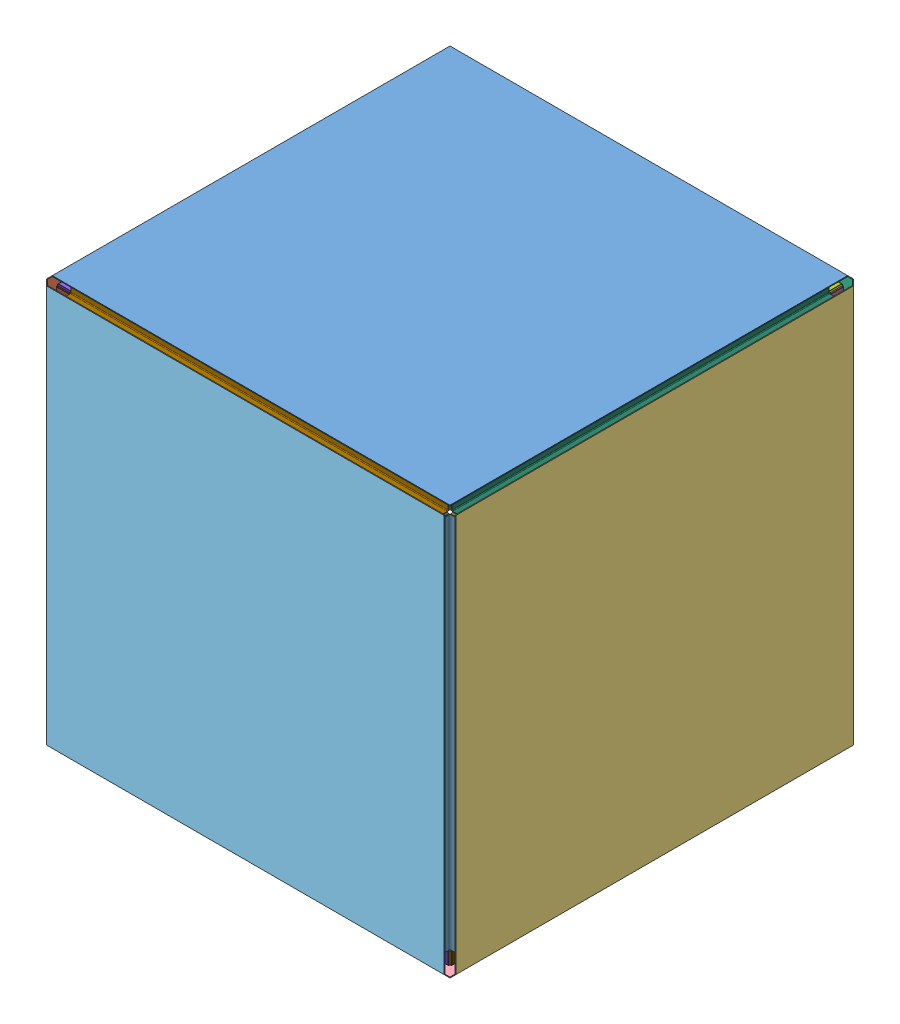
SolidWorks assembly cube_31, configuration cube31. Lengths in mm.
Overall size (770.25 770.25 770.25).
30 component instances, 30 part files, 93 mates.
Components (placement in the parent):
- pr^cube_31-28: pr^cube_31 [cube01] x (-1 0 0) z (0 0 1) size (748.03 1.59 748.03) (virtual)
- pg^cube_31-20: pg^cube_31 [cube01] x (0 -1 0) z (0 0 1) size (748.03 1.59 748.03) (virtual)
- po^cube_31-22: po^cube_31 [cube01] x (0 1 0) z (0 0 1) size (748.03 1.59 748.03) (virtual)
- py^cube_31-21: py^cube_31 [cube01] at origin size (748.03 1.59 748.03) (virtual)
- pc^cube_31-18: pc^cube_31 [cube01] x (-1 0 0) z (0 -1 0) size (748.03 1.59 748.03) (virtual)
- pb^cube_31-21: pb^cube_31 [cube01] x (-1 0 0) z (0 1 0) size (748.03 1.59 748.03) (virtual)
- br1^cube_31-49: br1^cube_31 [Default] at (0 358.14 -358.14) x (0 0 1) z (-1 0 0) size (50.8 50.8 709.17) (virtual)
- br2^cube_31-61: br2^cube_31 [Default] at (-358.14 358.14 0) size (50.8 50.8 709.17) (virtual)
- br3^cube_31-46: br3^cube_31 [Default] at (0 358.14 358.14) x (0 0 -1) z (1 0 0) size (50.8 50.8 709.17) (virtual)
- bg1^cube_31-47: bg1^cube_31 [Default] at (-358.14 -358.14 0) x (0 1 0) z (0 0 1) size (50.8 50.8 709.17) (virtual)
- bg2^cube_31-44: bg2^cube_31 [Default] at (-358.14 0 358.14) x (0 0 -1) z (0 1 0) size (50.8 50.8 709.17) (virtual)
- bg3^cube_31-40: bg3^cube_31 [Default] at (-358.14 0 -358.14) x (0 0 1) z (0 -1 0) size (50.8 50.8 709.17) (virtual)
- bo1^cube_31-42: bo1^cube_31 [Default] at (358.14 0 -358.14) x (0 0 1) z (0 1 0) size (50.8 50.8 709.17) (virtual)
- bo2^cube_31-46: bo2^cube_31 [Default] at (358.14 0 358.14) x (0 0 -1) z (0 -1 0) size (50.8 50.8 709.17) (virtual)
- bo3^cube_31-62: bo3^cube_31 [Default] at (358.14 358.14 0) x (0 -1 0) z (0 0 1) size (50.8 50.8 709.17) (virtual)
- by1^cube_31-41: by1^cube_31 [Default] at (0 -358.14 -358.14) x (0 0 1) z (1 0 0) size (50.8 50.8 709.17) (virtual)
- by2^cube_31-45: by2^cube_31 [Default] at (0 -358.14 358.14) x (0 0 -1) z (-1 0 0) size (50.8 50.8 709.17) (virtual)
- by3^cube_31-48: by3^cube_31 [Default] at (358.14 -358.14 0) x (-1 0 0) z (0 0 1) size (50.8 50.8 709.17) (virtual)
- dr1^cube_31-55: dr1^cube_31 [cube01] at (-382.9346 383.54 0) x (0 -1 0) z (0 0 1) size (26.01 26.01 767.09) (hidden, virtual)
- dr2^cube_31-37: dr2^cube_31 [cube01] at (0 383.54 382.9346) x (0 -1 0) z (1 0 0) size (26.01 26.01 767.09) (hidden, virtual)
- dr3^cube_31-33: dr3^cube_31 [cube01] at (0 383.54 -382.9346) x (0 -1 0) z (-1 0 0) size (26.01 26.01 767.09) (hidden, virtual)
- dg1^cube_31-38: dg1^cube_31 [cube01] at (-383.54 0 382.9346) x (1 0 0) z (0 1 0) size (26.01 26.01 767.09) (hidden, virtual)
- dg2^cube_31-41: dg2^cube_31 [cube01] at (-383.54 -382.9346 0) size (26.01 26.01 767.09) (hidden, virtual)
- dg3^cube_31-34: dg3^cube_31 [cube01] at (-383.54 0 -382.9346) x (1 0 0) z (0 -1 0) size (26.01 26.01 767.09) (hidden, virtual)
- do3^cube_31-47: do3^cube_31 [cube01] at (383.54 382.9346 0) x (-1 0 0) z (0 0 1) size (26.01 26.01 767.09) (hidden, virtual)
- do1^cube_31-36: do1^cube_31 [cube01] at (383.54 0 -382.9346) x (-1 0 0) z (0 1 0) size (26.01 26.01 767.09) (hidden, virtual)
- do2^cube_31-40: do2^cube_31 [cube01] at (383.54 0 382.9346) x (-1 0 0) z (0 -1 0) size (26.01 26.01 767.09) (hidden, virtual)
- dy1^cube_31-35: dy1^cube_31 [cube01] at (0 -383.54 -382.9346) x (0 1 0) z (1 0 0) size (26.01 26.01 767.09) (hidden, virtual)
- dy2^cube_31-39: dy2^cube_31 [cube01] at (0 -383.54 382.9346) x (0 1 0) z (-1 0 0) size (26.01 26.01 767.09) (hidden, virtual)
- dy3^cube_31-42: dy3^cube_31 [cube01] at (382.9346 -383.54 0) x (0 1 0) z (0 0 1) size (26.01 26.01 767.09) (hidden, virtual)
Mates (geometry in assembly coordinates):
- Coincident1: coincident anti-aligned: plane of pr^cube_31-28 through (374.015 383.54 -374.015) normal (0 -1 0); plane of br1^cube_31-49 through (-354.584 383.54 -358.14) normal (0 1 0)
- Coincident2: coincident anti-aligned: plane of pr^cube_31-28 through (374.015 383.54 -374.015) normal (0 -1 0); plane of br2^cube_31-61 through (-358.14 383.54 354.584) normal (0 1 0)
- Coincident3: coincident anti-aligned: plane of pr^cube_31-28 through (374.015 383.54 -374.015) normal (0 -1 0); plane of br3^cube_31-46 through (354.584 383.54 358.14) normal (0 1 0)
- Coincident4: coincident anti-aligned: plane of pr^cube_31-28 through (374.015 383.54 -374.015) normal (0 -1 0); plane of bo3^cube_31-62 through (358.14 383.54 354.584) normal (0 1 0)
- Coincident5: coincident anti-aligned: plane of pr^cube_31-28 through (374.015 383.54 -374.015) normal (0 -1 0); plane of dr3^cube_31-33 through (0 383.54 -766.4746) normal (0 1 0)
- Coincident6: coincident anti-aligned: plane of pr^cube_31-28 through (374.015 383.54 -374.015) normal (0 -1 0); plane of dr1^cube_31-55 through (-766.4746 383.54 0) normal (0 1 0)
- Coincident7: coincident anti-aligned: plane of pr^cube_31-28 through (374.015 383.54 -374.015) normal (0 -1 0); plane of do3^cube_31-47 through (-0.6054 383.54 0) normal (0 1 0)
- Coincident8: coincident anti-aligned: plane of pr^cube_31-28 through (374.015 383.54 -374.015) normal (0 -1 0); plane of dr2^cube_31-37 through (0 383.54 766.4746) normal (0 1 0)
- Coincident34: coincident anti-aligned: plane of pb^cube_31-21 through (374.015 -374.015 -383.54) normal (0 0 1); plane of by1^cube_31-41 through (354.584 -358.14 -383.54) normal (0 0 -1)
- Coincident35: coincident anti-aligned: plane of pb^cube_31-21 through (374.015 -374.015 -383.54) normal (0 0 1); plane of bo1^cube_31-42 through (358.14 354.584 -383.54) normal (0 0 -1)
- Coincident36: coincident anti-aligned: plane of pb^cube_31-21 through (374.015 -374.015 -383.54) normal (0 0 1); plane of br1^cube_31-49 through (-354.584 358.14 -383.54) normal (0 0 -1)
- Coincident37: coincident anti-aligned: plane of pb^cube_31-21 through (374.015 -374.015 -383.54) normal (0 0 1); plane of bg3^cube_31-40 through (-358.14 -354.584 -383.54) normal (0 0 -1)
- Coincident38: coincident anti-aligned: plane of pb^cube_31-21 through (374.015 -374.015 -383.54) normal (0 0 1); plane of dg3^cube_31-34 through (0.6054 0 -383.54) normal (0 0 -1)
- Coincident39: coincident anti-aligned: plane of pb^cube_31-21 through (374.015 -374.015 -383.54) normal (0 0 1); plane of dr3^cube_31-33 through (0 -0.6054 -383.54) normal (0 0 -1)
- Coincident40: coincident anti-aligned: plane of pb^cube_31-21 through (374.015 -374.015 -383.54) normal (0 0 1); plane of do1^cube_31-36 through (-0.6054 0 -383.54) normal (0 0 -1)
- Coincident41: coincident anti-aligned: plane of pb^cube_31-21 through (374.015 -374.015 -383.54) normal (0 0 1); plane of dy1^cube_31-35 through (0 0.6054 -383.54) normal (0 0 -1)
- Coincident42: coincident anti-aligned: plane of pc^cube_31-18 through (374.015 374.015 383.54) normal (0 0 -1); plane of bo2^cube_31-46 through (358.14 -354.584 383.54) normal (0 0 1)
- Coincident43: coincident anti-aligned: plane of pc^cube_31-18 through (374.015 374.015 383.54) normal (0 0 -1); plane of br3^cube_31-46 through (354.584 358.14 383.54) normal (0 0 1)
- Coincident44: coincident anti-aligned: plane of pc^cube_31-18 through (374.015 374.015 383.54) normal (0 0 -1); plane of bg2^cube_31-44 through (-358.14 354.584 383.54) normal (0 0 1)
- Coincident45: coincident anti-aligned: plane of pc^cube_31-18 through (374.015 374.015 383.54) normal (0 0 -1); plane of by2^cube_31-45 through (-354.584 -358.14 383.54) normal (0 0 1)
- Coincident46: coincident anti-aligned: plane of pc^cube_31-18 through (374.015 374.015 383.54) normal (0 0 -1); plane of do2^cube_31-40 through (-0.6054 0 383.54) normal (0 0 1)
- Coincident47: coincident anti-aligned: plane of pc^cube_31-18 through (374.015 374.015 383.54) normal (0 0 -1); plane of dy2^cube_31-39 through (0 0.6054 383.54) normal (0 0 1)
- Coincident48: coincident anti-aligned: plane of pc^cube_31-18 through (374.015 374.015 383.54) normal (0 0 -1); plane of dg1^cube_31-38 through (0.6054 0 383.54) normal (0 0 1)
- Coincident49: coincident anti-aligned: plane of pc^cube_31-18 through (374.015 374.015 383.54) normal (0 0 -1); plane of dr2^cube_31-37 through (0 -0.6054 383.54) normal (0 0 1)
- Coincident50: coincident anti-aligned: plane of pg^cube_31-20 through (-383.54 374.015 -374.015) normal (1 0 0); plane of bg3^cube_31-40 through (-383.54 -354.584 -358.14) normal (-1 0 0)
- Coincident51: coincident anti-aligned: plane of pg^cube_31-20 through (-383.54 374.015 -374.015) normal (1 0 0); plane of bg1^cube_31-47 through (-383.54 -358.14 354.584) normal (-1 0 0)
- Coincident52: coincident anti-aligned: plane of pg^cube_31-20 through (-383.54 374.015 -374.015) normal (1 0 0); plane of bg2^cube_31-44 through (-383.54 354.584 358.14) normal (-1 0 0)
- Coincident53: coincident anti-aligned: plane of pg^cube_31-20 through (-383.54 374.015 -374.015) normal (1 0 0); plane of dr1^cube_31-55 through (-383.54 -0.6054 0) normal (-1 0 0)
- Coincident54: coincident anti-aligned: plane of pg^cube_31-20 through (-383.54 374.015 -374.015) normal (1 0 0); plane of dg3^cube_31-34 through (-383.54 0 -766.4746) normal (-1 0 0)
- Coincident55: coincident anti-aligned: plane of pg^cube_31-20 through (-383.54 374.015 -374.015) normal (1 0 0); plane of dg2^cube_31-41 through (-383.54 -766.4746 0) normal (-1 0 0)
- Coincident56: coincident anti-aligned: plane of pg^cube_31-20 through (-383.54 374.015 -374.015) normal (1 0 0); plane of dg1^cube_31-38 through (-383.54 0 766.4746) normal (-1 0 0)
- Coincident99: coincident anti-aligned: plane of pg^cube_31-20 through (-383.54 374.015 -374.015) normal (1 0 0); plane of br2^cube_31-61 through (-383.54 358.14 354.584) normal (-1 0 0)
- Coincident57: coincident anti-aligned: plane of py^cube_31-21 through (-374.015 -383.54 -374.015) normal (0 1 0); plane of by3^cube_31-48 through (358.14 -383.54 354.584) normal (0 -1 0)
- Coincident58: coincident anti-aligned: plane of py^cube_31-21 through (-374.015 -383.54 -374.015) normal (0 1 0); plane of by2^cube_31-45 through (-354.584 -383.54 358.14) normal (0 -1 0)
- Coincident59: coincident anti-aligned: plane of py^cube_31-21 through (-374.015 -383.54 -374.015) normal (0 1 0); plane of bg1^cube_31-47 through (-358.14 -383.54 354.584) normal (0 -1 0)
- Coincident60: coincident anti-aligned: plane of py^cube_31-21 through (-374.015 -383.54 -374.015) normal (0 1 0); plane of by1^cube_31-41 through (354.584 -383.54 -358.14) normal (0 -1 0)
- Coincident61: coincident anti-aligned: plane of py^cube_31-21 through (-374.015 -383.54 -374.015) normal (0 1 0); plane of dy3^cube_31-42 through (766.4746 -383.54 0) normal (0 -1 0)
- Coincident62: coincident anti-aligned: plane of py^cube_31-21 through (-374.015 -383.54 -374.015) normal (0 1 0); plane of dy2^cube_31-39 through (0 -383.54 766.4746) normal (0 -1 0)
- Coincident63: coincident anti-aligned: plane of py^cube_31-21 through (-374.015 -383.54 -374.015) normal (0 1 0); plane of dg2^cube_31-41 through (0.6054 -383.54 0) normal (0 -1 0)
- Coincident64: coincident anti-aligned: plane of py^cube_31-21 through (-374.015 -383.54 -374.015) normal (0 1 0); plane of dy1^cube_31-35 through (0 -383.54 -766.4746) normal (0 -1 0)
- Coincident65: coincident anti-aligned: plane of po^cube_31-22 through (383.54 -374.015 -374.015) normal (-1 0 0); plane of bo1^cube_31-42 through (383.54 354.584 -358.14) normal (1 0 0)
- Coincident66: coincident anti-aligned: plane of po^cube_31-22 through (383.54 -374.015 -374.015) normal (-1 0 0); plane of by3^cube_31-48 through (383.54 -358.14 354.584) normal (1 0 0)
- Coincident67: coincident anti-aligned: plane of po^cube_31-22 through (383.54 -374.015 -374.015) normal (-1 0 0); plane of bo2^cube_31-46 through (383.54 -354.584 358.14) normal (1 0 0)
- Coincident68: coincident anti-aligned: plane of po^cube_31-22 through (383.54 -374.015 -374.015) normal (-1 0 0); plane of bo3^cube_31-62 through (383.54 358.14 354.584) normal (1 0 0)
- Coincident69: coincident anti-aligned: plane of po^cube_31-22 through (383.54 -374.015 -374.015) normal (-1 0 0); plane of do2^cube_31-40 through (383.54 0 766.4746) normal (1 0 0)
- Coincident70: coincident anti-aligned: plane of po^cube_31-22 through (383.54 -374.015 -374.015) normal (-1 0 0); plane of do3^cube_31-47 through (383.54 766.4746 0) normal (1 0 0)
- Coincident71: coincident anti-aligned: plane of po^cube_31-22 through (383.54 -374.015 -374.015) normal (-1 0 0); plane of do1^cube_31-36 through (383.54 0 -766.4746) normal (1 0 0)
- Coincident72: coincident anti-aligned: plane of po^cube_31-22 through (383.54 -374.015 -374.015) normal (-1 0 0); plane of dy3^cube_31-42 through (383.54 0.6054 0) normal (1 0 0)
- Coincident73: coincident aligned: plane of assembly through (0 0 0) normal (0 0 1); plane of dy3^cube_31-42 through (382.9346 -383.54 0) normal (0 0 1)
- Coincident74: coincident aligned: plane of assembly through (0 0 0) normal (0 0 1); plane of by3^cube_31-48 through (358.14 -358.14 0) normal (0 0 1)
- Coincident75: coincident aligned: plane of assembly through (0 0 0) normal (0 0 1); plane of bo3^cube_31-62 through (358.14 358.14 0) normal (0 0 1)
- Coincident76: coincident aligned: plane of assembly through (0 0 0) normal (0 0 1); plane of do3^cube_31-47 through (383.54 382.9346 0) normal (0 0 1)
- Coincident77: coincident aligned: plane of assembly through (0 0 0) normal (0 0 1); plane of dg2^cube_31-41 through (-383.54 -382.9346 0) normal (0 0 1)
- Coincident78: coincident aligned: plane of assembly through (0 0 0) normal (0 0 1); plane of bg1^cube_31-47 through (-358.14 -358.14 0) normal (0 0 1)
- Coincident79: coincident aligned: plane of assembly through (0 0 0) normal (0 0 1); plane of dr1^cube_31-55 through (-382.9346 383.54 0) normal (0 0 1)
- Coincident80: coincident aligned: plane of assembly through (0 0 0) normal (0 0 1); plane of br2^cube_31-61 through (-358.14 358.14 0) normal (0 0 1)
- Coincident81: coincident aligned: plane of assembly through (0 0 0) normal (0 1 0); plane of bo1^cube_31-42 through (358.14 0 -358.14) normal (0 1 0)
- Coincident82: coincident aligned: plane of assembly through (0 0 0) normal (0 1 0); plane of py^cube_31-21 through (0 0 0) normal (0 1 0)
- Coincident83: coincident aligned: plane of assembly through (0 0 0) normal (0 1 0); plane of do1^cube_31-36 through (383.54 0 -382.9346) normal (0 1 0)
- Coincident84: coincident anti-aligned: plane of assembly through (0 0 0) normal (0 1 0); plane of bg3^cube_31-40 through (-358.14 0 -358.14) normal (0 -1 0)
- Coincident85: coincident anti-aligned: plane of assembly through (0 0 0) normal (0 1 0); plane of dg3^cube_31-34 through (-383.54 0 -382.9346) normal (0 -1 0)
- Coincident86: coincident aligned: plane of assembly through (0 0 0) normal (0 1 0); plane of dg1^cube_31-38 through (-383.54 0 382.9346) normal (0 1 0)
- Coincident87: coincident aligned: plane of assembly through (0 0 0) normal (0 1 0); plane of bg2^cube_31-44 through (-358.14 0 358.14) normal (0 1 0)
- Coincident88: coincident anti-aligned: plane of assembly through (0 0 0) normal (0 1 0); plane of bo2^cube_31-46 through (358.14 0 358.14) normal (0 -1 0)
- Coincident89: coincident anti-aligned: plane of assembly through (0 0 0) normal (0 1 0); plane of do2^cube_31-40 through (383.54 0 382.9346) normal (0 -1 0)
- Coincident90: coincident anti-aligned: plane of assembly through (0 0 0) normal (1 0 0); plane of by2^cube_31-45 through (0 -358.14 358.14) normal (-1 0 0)
- Coincident91: coincident anti-aligned: plane of assembly through (0 0 0) normal (1 0 0); plane of dy2^cube_31-39 through (0 -383.54 382.9346) normal (-1 0 0)
- Coincident92: coincident aligned: plane of assembly through (0 0 0) normal (1 0 0); plane of pg^cube_31-20
- Coincident93: coincident aligned: plane of assembly through (0 0 0) normal (1 0 0); plane of dr2^cube_31-37 through (0 383.54 382.9346) normal (1 0 0)
- Coincident94: coincident aligned: plane of assembly through (0 0 0) normal (1 0 0); plane of br3^cube_31-46 through (0 358.14 358.14) normal (1 0 0)
- Coincident95: coincident anti-aligned: plane of assembly through (0 0 0) normal (1 0 0); plane of dr3^cube_31-33 through (0 383.54 -382.9346) normal (-1 0 0)
- Coincident96: coincident anti-aligned: plane of assembly through (0 0 0) normal (1 0 0); plane of br1^cube_31-49 through (0 358.14 -358.14) normal (-1 0 0)
- Coincident97: coincident aligned: plane of assembly through (0 0 0) normal (1 0 0); plane of by1^cube_31-41 through (0 -358.14 -358.14) normal (1 0 0)
- Coincident98: coincident aligned: plane of assembly through (0 0 0) normal (1 0 0); plane of dy1^cube_31-35 through (0 -383.54 -382.9346) normal (1 0 0)
- Coincident100: coincident anti-aligned: plane of pr^cube_31-28; plane of assembly through (0 0 0) normal (1 0 0)
- Coincident101: coincident aligned: plane of pr^cube_31-28 through (0 0 0) normal (0 0 1); plane of assembly through (0 0 0) normal (0 0 1)
- Coincident102: coincident anti-aligned: plane of pr^cube_31-28; plane of assembly through (0 0 0) normal (0 1 0)
- Coincident106: coincident anti-aligned: plane of pg^cube_31-20; plane of assembly through (0 0 0) normal (0 1 0)
- Coincident107: coincident aligned: plane of pg^cube_31-20; plane of assembly through (0 0 0) normal (1 0 0)
- Coincident108: coincident aligned: plane of pg^cube_31-20 through (0 0 0) normal (0 0 1); plane of assembly through (0 0 0) normal (0 0 1)
- Coincident109: coincident aligned: plane of py^cube_31-21 through (0 0 0) normal (0 0 1); plane of assembly through (0 0 0) normal (0 0 1)
- Coincident110: coincident aligned: plane of py^cube_31-21 through (0 0 0) normal (0 1 0); plane of assembly through (0 0 0) normal (0 1 0)
- Coincident111: coincident aligned: plane of py^cube_31-21 through (0 0 0) normal (1 0 0); plane of assembly through (0 0 0) normal (1 0 0)
- Coincident112: coincident aligned: plane of po^cube_31-22 through (0 0 0) normal (0 0 1); plane of assembly through (0 0 0) normal (0 0 1)
- Coincident113: coincident anti-aligned: plane of po^cube_31-22; plane of assembly through (0 0 0) normal (1 0 0)
- Coincident114: coincident aligned: plane of po^cube_31-22; plane of assembly through (0 0 0) normal (0 1 0)
- Coincident115: coincident anti-aligned: plane of pc^cube_31-18 through (0 0 0) normal (0 -1 0); plane of assembly through (0 0 0) normal (0 1 0)
- Coincident116: coincident anti-aligned: plane of pc^cube_31-18; plane of assembly through (0 0 0) normal (0 0 1)
- Coincident117: coincident anti-aligned: plane of pc^cube_31-18; plane of assembly through (0 0 0) normal (1 0 0)
- Coincident118: coincident aligned: plane of pb^cube_31-21 through (0 0 0) normal (0 1 0); plane of assembly through (0 0 0) normal (0 1 0)
- Coincident119: coincident aligned: plane of pb^cube_31-21; plane of assembly through (0 0 0) normal (0 0 1)
- Coincident120: coincident anti-aligned: line of pb^cube_31-21 through (0.8731 -0.8731 0) axis (0 0 -1); sketch_entity of pr^cube_31-28; plane of pb^cube_31-21 through (374.015 -374.015 -385.1275) normal (0 0 -1); plane of py^cube_31-21 through (-374.015 -385.1275 -374.015) normal (0 -1 0)
- cyan_cut: unknown: unknown of pc^cube_31-18; plane of pc^cube_31-18 through (374.015 374.015 385.1275) normal (0 0 1); plane of pg^cube_31-20 through (-385.1275 374.015 -374.015) normal (-1 0 0); plane of po^cube_31-22 through (385.1275 -374.015 -374.015) normal (1 0 0)
